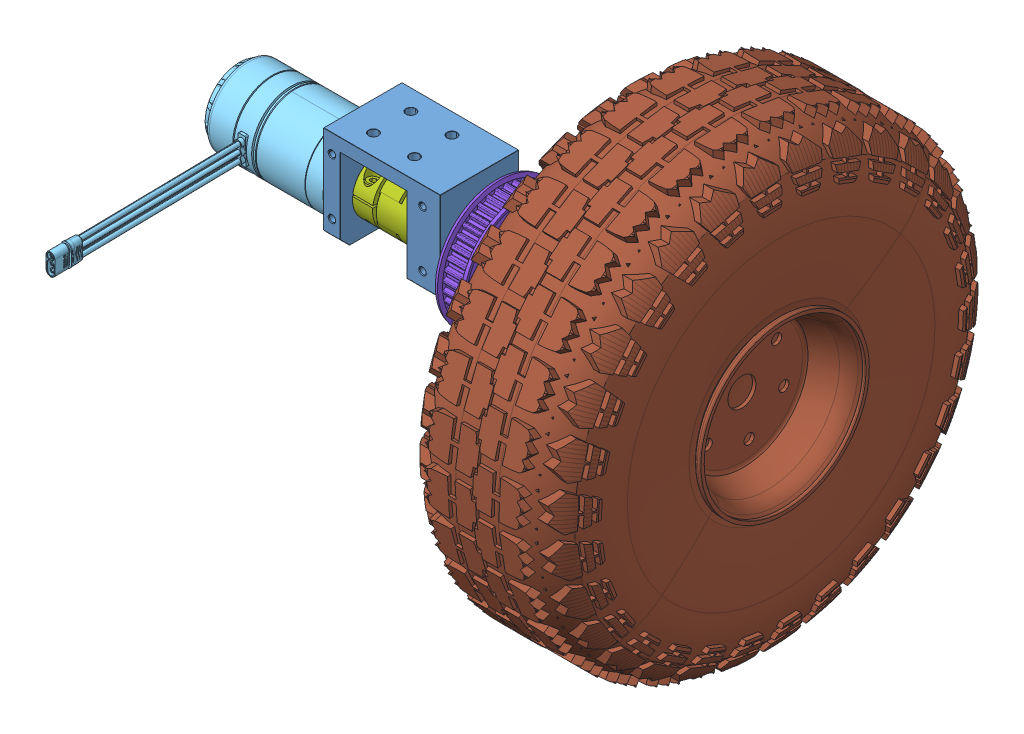
SolidWorks assembly 轮胎模组, configuration 默认. Lengths in mm.
Overall size (297.23 341.76 341.72).
20 component instances, 12 part files, 41 mates.
Components (placement in the parent):
- m3508-1: m3508 [Default] at (-12.228 0.9134 62.5) size (62.5 52.5 42)
- deep groove ball bearings gb-1: deep groove ball bearings gb [Rolling bearings 6000 GB 276-94] at (6.9178 -9.2089 62.5) size (8 26 26)
- deep groove ball bearings gb-2: deep groove ball bearings gb [Rolling bearings 6000 GB 276-94] at (14.9178 -9.2089 62.5) x (1 0 0) z (0 0.136617 0.990624) size (8 26 26)
- plain washers for clevis pins gb-1: plain washers for clevis pins gb [GB_ROUND_WASHERS_TYPE7 3] at (19.7178 1.5391 73.248) x (0 0 -1) z (1 0 0) size (6 6 0.8)
- plain washers for clevis pins gb-2: plain washers for clevis pins gb [GB_ROUND_WASHERS_TYPE7 3] at (19.7178 1.5391 51.752) x (0 0 -1) z (1 0 0) size (6 6 0.8)
- plain washers for clevis pins gb-3: plain washers for clevis pins gb [GB_ROUND_WASHERS_TYPE7 3] at (19.7178 -20.4006 72.7853) x (0 0 -1) z (1 0 0) size (6 6 0.8)
- plain washers for clevis pins gb-4: plain washers for clevis pins gb [GB_ROUND_WASHERS_TYPE7 3] at (19.7178 -19.4942 51.3083) x (0 0 -1) z (1 0 0) size (6 6 0.8)
- hexagon socket head cap screws gb-1: hexagon socket head cap screws gb [GB_FASTENER_SCREWS_HSHCS M3X8-N] at (22.7178 1.5391 73.248) x (-1 0 0) z (0 0.924225 0.381849) size (11 5.5 5.5)
- hexagon socket head cap screws gb-2: hexagon socket head cap screws gb [GB_FASTENER_SCREWS_HSHCS M3X8-N] at (22.7178 1.5391 51.752) x (-1 0 0) z (0 0.924225 0.381849) size (11 5.5 5.5)
- hexagon socket head cap screws gb-3: hexagon socket head cap screws gb [GB_FASTENER_SCREWS_HSHCS M3X8-N] at (22.7178 -20.4006 72.7853) x (-1 0 0) z (0 0.924225 0.381849) size (11 5.5 5.5)
- hexagon socket head cap screws gb-4: hexagon socket head cap screws gb [GB_FASTENER_SCREWS_HSHCS M3X8-N] at (22.7178 -19.4942 51.3083) x (-1 0 0) z (0 0.924225 0.381849) size (11 5.5 5.5)
- RoboMaster M3508直流无刷减速电-1: RoboMaster M3508直流无刷减速电 [默认] at (-130.0232 -5.7399 80.5249) x (0 -0.958889 0.283782) z (1 0 0) size (63.71 141.17 98.4)
- 轴-1: 轴 [默认] at (18.9178 -9.2089 62.5) x (0 0.982488 0.186325) z (0 -0.186325 0.982488) size (16 128 16)
- CPJCK30-RD-10-10-1: CPJCK30-RD-10-10 [Default] at (-34.3322 -9.2089 62.5) x (1 0 0) z (0 0.124503 0.992219) size (35 30 30)
- 同步轮-1: 同步轮 [Default] at (28.0178 -9.2089 62.5) size (16 67 67)
- 平键5x5x35-1: 平键5x5x35 [默认] at (94.4178 -1.8402 63.8974) x (0 -0.186325 0.982488) z (0 -0.982488 -0.186325) size (5 41 5)
- 法兰-1: 法兰 [默认] at (113.9178 -9.2089 62.5) x (0 0.186325 -0.982488) z (1 0 0) size (60 60 41)
- 10寸充气轮-1: 10寸充气轮 [Default] at (181.1138 -179.9795 79.9579) x (0 0.631528 -0.775353) z (1 0 0) size (242.76 243.05 91.75)
- circlips for shaft--type a large gb-1: circlips for shaft--type a large gb [GB_CONNECTING_PIECE_RING_RRA 16] at (28.0178 -8.6289 62.5) x (0 0 -1) z (1 0 0) size (18.2 20.68 1)
- circlips for shaft--type a large gb-2: circlips for shaft--type a large gb [GB_CONNECTING_PIECE_RING_RRA 16] at (44.0178 -8.6289 62.5) x (0 0 1) z (-1 0 0) size (18.2 20.68 1)
Mates (geometry in assembly coordinates):
- Concentric1: concentric: cylinder of assembly; cylinder of assembly; cylinder of m3508-1 through (2.9178 -9.2089 62.5) axis (1 0 0) radius 13; cylinder of deep groove ball bearings gb-1 through (-1.7928 -9.2089 62.5) axis (-1 0 0) radius 13
- Coincident1: coincident: plane of assembly; plane of assembly; plane of m3508-1 through (2.9178 -9.2089 62.5) normal (1 0 0); plane of deep groove ball bearings gb-1 through (2.9178 3.7911 62.5) normal (-1 0 0)
- Concentric2: concentric: cylinder of assembly; cylinder of assembly; cylinder of m3508-1 through (2.9178 -9.2089 62.5) axis (1 0 0) radius 13; cylinder of deep groove ball bearings gb-2 through (6.2072 -9.2089 62.5) axis (-1 0 0) radius 13
- Coincident2: coincident: plane of assembly; plane of assembly; plane of deep groove ball bearings gb-1 through (10.9178 3.7911 62.5) normal (1 0 0); plane of deep groove ball bearings gb-2 through (10.9178 3.6692 60.724) normal (-1 0 0)
- Concentric31: concentric: cone of assembly; cylinder of assembly; cone of m3508-1 through (18.3928 1.5391 73.248) axis (-1 0 0); cylinder of plain washers for clevis pins gb-1 through (18.9178 1.5391 73.248) axis (1 0 0) radius 1.57
- Coincident31: coincident: plane of assembly; plane of assembly; plane of m3508-1 through (18.9178 22.2911 83.5) normal (1 0 0); plane of plain washers for clevis pins gb-1 through (18.9178 1.5391 73.248) normal (-1 0 0)
- Concentric41: concentric: cone of assembly; cylinder of assembly; cone of m3508-1 through (18.3928 1.5391 51.752) axis (-1 0 0); cylinder of plain washers for clevis pins gb-2 through (18.9178 1.5391 51.752) axis (1 0 0) radius 1.57
- Coincident41: coincident: plane of assembly; plane of assembly; plane of m3508-1 through (18.9178 22.2911 83.5) normal (1 0 0); plane of plain washers for clevis pins gb-2 through (18.9178 1.5391 51.752) normal (-1 0 0)
- Concentric51: concentric: cone of assembly; cylinder of assembly; cone of m3508-1 through (18.3928 -20.4006 72.7853) axis (-1 0 0); cylinder of plain washers for clevis pins gb-3 through (18.9178 -20.4006 72.7853) axis (1 0 0) radius 1.57
- Coincident51: coincident: plane of assembly; plane of assembly; plane of m3508-1 through (18.9178 22.2911 83.5) normal (1 0 0); plane of plain washers for clevis pins gb-3 through (18.9178 -20.4006 72.7853) normal (-1 0 0)
- Concentric61: concentric: cone of assembly; cylinder of assembly; cone of m3508-1 through (18.3928 -19.4942 51.3083) axis (-1 0 0); cylinder of plain washers for clevis pins gb-4 through (18.9178 -19.4942 51.3083) axis (1 0 0) radius 1.57
- Coincident61: coincident: plane of assembly; plane of assembly; plane of m3508-1 through (18.9178 22.2911 83.5) normal (1 0 0); plane of plain washers for clevis pins gb-4 through (18.9178 -19.4942 51.3083) normal (-1 0 0)
- Concentric71: concentric: cylinder of assembly; cylinder of assembly; cylinder of plain washers for clevis pins gb-1 through (18.9178 1.5391 73.248) axis (1 0 0) radius 3; cylinder of hexagon socket head cap screws gb-1 through (11.7178 1.5391 73.248) axis (1 0 0) radius 1.5
- Coincident71: coincident: plane of assembly; plane of assembly; plane of plain washers for clevis pins gb-1 through (19.7178 1.5391 73.248) normal (1 0 0); plane of hexagon socket head cap screws gb-1 through (19.7178 1.5391 73.248) normal (-1 0 0)
- Concentric81: concentric: cylinder of assembly; cylinder of assembly; cylinder of plain washers for clevis pins gb-2 through (18.9178 1.5391 51.752) axis (1 0 0) radius 3; cylinder of hexagon socket head cap screws gb-2 through (11.7178 1.5391 51.752) axis (1 0 0) radius 1.5
- Coincident81: coincident: plane of assembly; plane of assembly; plane of plain washers for clevis pins gb-2 through (19.7178 1.5391 51.752) normal (1 0 0); plane of hexagon socket head cap screws gb-2 through (19.7178 1.5391 51.752) normal (-1 0 0)
- Concentric91: concentric: cylinder of assembly; cylinder of assembly; cylinder of plain washers for clevis pins gb-3 through (18.9178 -20.4006 72.7853) axis (1 0 0) radius 1.57; cylinder of hexagon socket head cap screws gb-3 through (11.7178 -20.4006 72.7853) axis (1 0 0) radius 1.5
- Coincident91: coincident: plane of assembly; plane of assembly; plane of plain washers for clevis pins gb-3 through (19.7178 -20.4006 72.7853) normal (1 0 0); plane of hexagon socket head cap screws gb-3 through (19.7178 -20.4006 72.7853) normal (-1 0 0)
- Concentric101: concentric: cylinder of assembly; cylinder of assembly; cylinder of plain washers for clevis pins gb-4 through (18.9178 -19.4942 51.3083) axis (1 0 0) radius 1.57; cylinder of hexagon socket head cap screws gb-4 through (11.7178 -19.4942 51.3083) axis (1 0 0) radius 1.5
- Coincident101: coincident: plane of assembly; plane of assembly; plane of plain washers for clevis pins gb-4 through (19.7178 -19.4942 51.3083) normal (1 0 0); plane of hexagon socket head cap screws gb-4 through (19.7178 -19.4942 51.3083) normal (-1 0 0)
- Coincident102: coincident: plane of assembly; plane of assembly; plane of m3508-1 through (-43.5822 22.2911 83.5) normal (-1 0 0); plane of RoboMaster M3508直流无刷减速电-1 through (-43.5822 -0.9847 72.5679) normal (1 0 0)
- Concentric102: concentric: cylinder of assembly; cylinder of assembly; cylinder of m3508-1 through (-34.5822 -9.2089 62.5) axis (-1 0 0) radius 13.05; cylinder of RoboMaster M3508直流无刷减速电-1 through (-16.2822 -9.2089 62.5) axis (1 0 0) radius 5
- Concentric103: concentric: cylinder of assembly; cylinder of assembly; cylinder of deep groove ball bearings gb-2 through (7.9464 -9.2089 62.5) axis (-1 0 0) radius 5; cylinder of 轴-1 through (-14.0822 -9.2089 62.5) axis (1 0 0) radius 5
- Coincident103: coincident: plane of assembly; plane of assembly; plane of deep groove ball bearings gb-2 through (18.9178 -4.2558 61.8169) normal (1 0 0); plane of 轴-1 through (18.9178 -9.2089 62.5) normal (-1 0 0)
- Concentric104: concentric: cylinder of assembly; cylinder of assembly; cylinder of 轴-1 through (-14.0822 -9.2089 62.5) axis (1 0 0) radius 5; cylinder of CPJCK30-RD-10-10-1 through (0.6678 -9.2089 62.5) axis (-1 0 0) radius 5
- Width1: width: plane of assembly; plane of assembly; plane of assembly; plane of assembly; plane of m3508-1 through (0.9178 15.2911 41.5) normal (-1 0 0); plane of m3508-1 through (-34.5822 -34.5225 41.5) normal (1 0 0); plane of CPJCK30-RD-10-10-1 through (0.6678 -4.2478 61.8775) normal (1 0 0); plane of CPJCK30-RD-10-10-1 through (-34.3322 5.4263 60.6636) normal (-1 0 0)
- Concentric105: concentric: cylinder of assembly; cylinder of assembly; cylinder of 轴-1 through (113.9178 -9.2089 62.5) axis (-1 0 0) radius 8; cylinder of 同步轮-1 through (44.0178 -9.2089 62.5) axis (-1 0 0) radius 8
- Coincident104: coincident: plane of assembly; plane of assembly; plane of 轴-1 through (28.0178 -9.2089 62.5) normal (-1 0 0); plane of 同步轮-1 through (28.0178 -9.2089 62.5) normal (-1 0 0)
- Coincident105: coincident: plane of assembly; plane of assembly; plane of 轴-1 through (395.1486 -2.2085 66.3722) normal (0 0.186325 -0.982488); plane of 平键5x5x35-1 through (73.9178 0.1502 66.8195) normal (0 -0.186325 0.982488)
- Concentric106: concentric: cylinder of assembly; cylinder of assembly; cylinder of 轴-1 through (76.4178 -9.2089 62.5) axis (0 -0.982488 -0.186325) radius 2.5; cylinder of 平键5x5x35-1 through (76.4178 -1.8402 63.8974) axis (0 -0.982488 -0.186325) radius 2.5
- Coincident106: coincident: plane of assembly; plane of assembly; plane of 轴-1 through (395.1486 -4.7623 65.8878) normal (0 0.982488 0.186325); plane of 平键5x5x35-1 through (73.9178 -3.8307 60.9754) normal (0 -0.982488 -0.186325)
- Width2: width: plane of assembly; plane of assembly; plane of assembly; plane of assembly; plane of 法兰-1 through (113.9178 -1.2768 61.4597) normal (0 -0.186325 0.982488); plane of 法兰-1 through (113.9178 0.4449 66.8754) normal (0 0.186325 -0.982488); plane of 平键5x5x35-1 through (73.9178 1.0818 61.907) normal (0 0.186325 -0.982488); plane of 平键5x5x35-1 through (73.9178 0.1502 66.8195) normal (0 -0.186325 0.982488)
- Concentric107: concentric: cylinder of assembly; cylinder of assembly; cylinder of 轴-1 through (113.9178 -9.2089 62.5) axis (-1 0 0) radius 8; cylinder of 法兰-1 through (113.9178 -9.2089 62.5) axis (-1 0 0) radius 8
- Coincident107: coincident: plane of assembly; plane of assembly; plane of 轴-1 through (113.9178 -9.2089 62.5) normal (1 0 0); plane of 法兰-1 through (113.9178 -9.2089 62.5) normal (1 0 0)
- Coincident108: coincident: plane of assembly; plane of assembly; plane of 法兰-1 through (113.9178 -9.2089 62.5) normal (1 0 0); plane of 10寸充气轮-1 through (113.9178 -9.2089 62.5) normal (-1 0 0)
- Concentric108: concentric: cylinder of assembly; cylinder of assembly; cylinder of 法兰-1 through (113.9178 -9.2089 62.5) axis (1 0 0) radius 16; cylinder of 10寸充气轮-1 through (116.9642 -9.2089 62.5) axis (-1 0 0) radius 7.5
- Concentric109: concentric: cylinder of assembly; cylinder of assembly; cylinder of 法兰-1 through (113.9188 6.4536 44.3153) axis (-1 0 0) radius 2.75; cylinder of 10寸充气轮-1 through (132.8178 6.4536 44.3153) axis (-1 0 0) radius 2.75
- Concentric1101: concentric: cylinder of assembly; cylinder of assembly; cylinder of 轴-1 through (28.0178 -9.2089 62.5) axis (-1 0 0) radius 7.6; cylinder of circlips for shaft--type a large gb-1 through (27.0178 -9.2089 62.5) axis (1 0 0) radius 7.35
- Coincident1091: coincident: plane of assembly; plane of assembly; plane of 轴-1 through (28.0178 -9.2089 62.5) normal (-1 0 0); plane of circlips for shaft--type a large gb-1 through (28.0178 -9.2089 62.5) normal (1 0 0)
- Concentric1111: concentric: cylinder of assembly; cylinder of assembly; cylinder of 轴-1 through (45.1178 -9.2089 62.5) axis (-1 0 0) radius 7.6; cylinder of circlips for shaft--type a large gb-2 through (45.0178 -9.2089 62.5) axis (-1 0 0) radius 7.35
- Coincident1101: coincident: plane of assembly; plane of assembly; plane of 轴-1 through (44.0178 -9.2089 62.5) normal (1 0 0); plane of circlips for shaft--type a large gb-2 through (44.0178 -9.2089 62.5) normal (-1 0 0)
